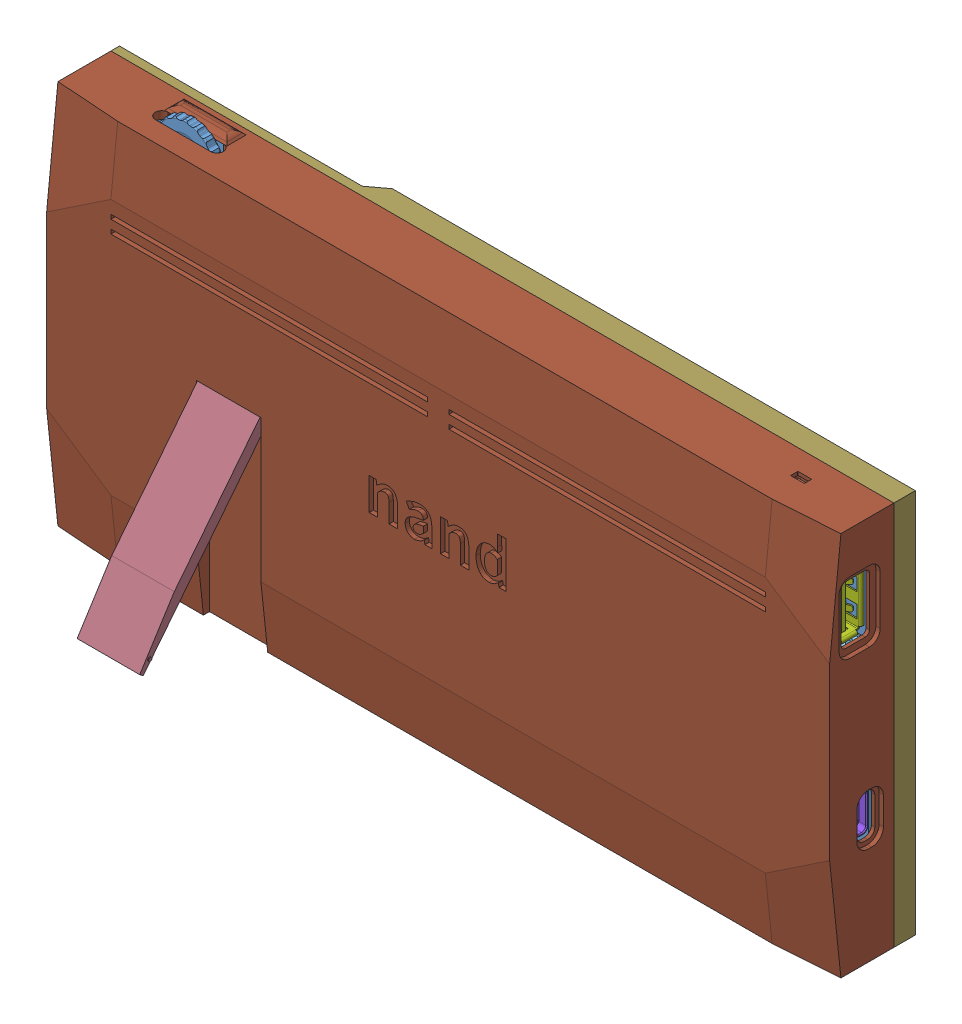
SolidWorks assembly model01, configuration 默认. Lengths in mm.
Overall size (182.71 95.18 52.67).
146 component instances, 34 part files, 28 mates.
Components (placement in the parent):
- Copy of CTR_PAD.step-1: Copy of CTR_PAD.step [默认] at (14.9481 50.9273 157.9259) size (178.7 93.18 19.65)
  - Board.step-1: Board.step [默认] at origin size (178.7 87.58 1.9)
    - Open CASCADE STEP translator 6.8 1.1.1.step-1: Open CASCADE STEP translator 6.8 1.1.1.step [默认] at (0 0 -1.9037) size (178.7 87.58 1.9)
  - K1_1.step-1: K1_1.step [默认] at origin size (7.8 3.6 3.5)
    - User_Library-E-Switch_-_TL3330AF130QG_(Tact_Switch,_SMD).step-1: User_Library-E-Switch_-_TL3330AF130QG_(Tact_Switch,_SMD).step [默认] at (168.6 -0.394 0) x (-1 0 0) z (0 1 0) size (7.8 3.5 3.6)
  - JP4.step-1: JP4.step [默认] at origin size (5.19 12.65 3.4)
    - MOLEX1.25-WS-6P.step-1: MOLEX1.25-WS-6P.step [默认] at (176.345 -30.9118 0) x (0 1 0) z (0 0 1) size (12.65 5.19 3.4)
      - MOLEX1.25-WS-____.step-1: MOLEX1.25-WS-____.step [默认] at (3.125 1.89 1.375) size (0.32 4.2 1.72)
      - MOLEX1.25-WS-____.step-2: MOLEX1.25-WS-____.step [默认] at (1.875 1.89 1.375) size (0.32 4.2 1.72)
      - MOLEX1.25-WS-____.step-3: MOLEX1.25-WS-____.step [默认] at (0.625 1.89 1.375) size (0.32 4.2 1.72)
      - MOLEX1.25-WS-____.step-4: MOLEX1.25-WS-____.step [默认] at (-0.625 1.89 1.375) size (0.32 4.2 1.72)
      - MOLEX1.25-WS-____.step-5: MOLEX1.25-WS-____.step [默认] at (-1.875 1.89 1.375) size (0.32 4.2 1.72)
      - MOLEX1.25-WS-____.step-6: MOLEX1.25-WS-____.step [默认] at (-3.125 1.89 1.375) size (0.32 4.2 1.72)
      - LOGO_0.25.step-1: LOGO_0.25.step [默认] at (3.4 -1.1304 0.195) size (0.75 0.87 0.01)
      - MOLEX1.25-WS-6P-0.step-1: MOLEX1.25-WS-6P-0.step [默认] at origin size (12.65 4.2 3.4)
  - USB1.step-1: USB1.step [默认] at origin size (14.7 15.5 7.95)
    - USB_A_______-__-2.step-1: USB_A_______-__-2.step [默认] at (168.4838 -16.002 0) x (0 1 0) z (0 0 1) size (15.5 14.7 7.95)
      - LOGO_.step-1: LOGO_.step [默认] at (0.0236 -0.0345 0.196) x (-1 0 0) z (0 0 -1) size (1.2 1.38 0.01)
      - USB_A_______-__-2-1.step-1: USB_A_______-__-2-1.step [默认] at origin size (15.5 14.7 7.95)
  - U8.step-1: U8.step [默认] at origin size (7.9 8.94 4.2)
    - USB_Type_C_Port_(SMD_Type)_RGB15724527.step-1: USB_Type_C_Port_(SMD_Type)_RGB15724527.step [默认] at (171.3143 -58.97 1.651) x (0 1 0) z (0 0 -1) size (8.94 7.9 4.2)
  - JP2.step-1: JP2.step [默认] at origin size (0.51 6.25 12)
    - DJ610-4.8x0.5x14.step-1: DJ610-4.8x0.5x14.step [默认] at (155.879 -80.1986 -1.9037) x (0 1 0) z (0 0 -1) size (6.25 0.51 12)
      - DJ610-4.8x0.5x14-2.step-1: DJ610-4.8x0.5x14-2.step [默认] at origin size (6.25 0.51 12)
      - LOGO_0.1.step-1: LOGO_0.1.step [默认] at (-0.0714 0.0198 0.048) size (0.3 0.35 0)
  - JP3.step-1: JP3.step [默认] at origin size (0.51 6.25 12)
    - DJ610-4.8x0.5x14.step-1: DJ610-4.8x0.5x14.step [默认] at (145.719 -80.1986 -1.9037) x (0 1 0) z (0 0 -1) size (6.25 0.51 12)
      - DJ610-4.8x0.5x14-2.step-1: DJ610-4.8x0.5x14-2.step [默认] at origin size (6.25 0.51 12)
      - LOGO_0.1.step-1: LOGO_0.1.step [默认] at (-0.0714 0.0198 0.048) size (0.3 0.35 0)
  - Designator10.step-1: Designator10.step [默认] at origin size (6.5 7.3 13.51)
    - SMA-KE-LI.step-1: SMA-KE-LI.step [默认] at (110.2469 -80.1989 -1.9037) x (-1 0 0) z (0 0 -1) size (6.5 7.3 13.5)
      - SMA-KE-LI-3.step-1: SMA-KE-LI-3.step [默认] at origin size (6.5 7.3 13.5)
      - LOGO_0.25-4.step-1: LOGO_0.25-4.step [默认] at (0.0036 0.0616 -3.1525) size (0.75 0.87 0.01)
  - Designator9.step-1: Designator9.step [默认] at origin size (6.5 7.3 13.51)
    - SMA-KE-LI.step-1: SMA-KE-LI.step [默认] at (82.0269 -80.1369 -1.9037) x (-1 0 0) z (0 0 -1) size (6.5 7.3 13.5)
      - SMA-KE-LI-3.step-1: SMA-KE-LI-3.step [默认] at origin size (6.5 7.3 13.5)
      - LOGO_0.25-4.step-1: LOGO_0.25-4.step [默认] at (0.0036 0.0616 -3.1525) size (0.75 0.87 0.01)
  - R3.step-1: R3.step [默认] at origin size (1.6 0.8 0.4)
    - R_0603.step-1: R_0603.step [默认] at (50.1906 -13.906 -1.9037) x (-1 0 0) z (0 0 -1) size (1.6 0.8 0.4)
      - R_0603-5.step-1: R_0603-5.step [默认] at origin size (1.6 0.8 0.4)
      - LOGO_-6.step-1: LOGO_-6.step [默认] at (0.0001 0.0322 -0.0016) x (-1 0 0) z (0 0 -1) size (0.48 0.55 0)
  - KEY4.step-1: KEY4.step [默认] at origin size (10.71 10 7.1)
    - 43447.step-1: 43447.step [默认] at (38.778 -26.673 -1.9037) x (1 0 0) z (0 1 0) size (10.71 7.1 10)
  - KEY3.step-1: KEY3.step [默认] at origin size (10.71 10 7.1)
    - 43447.step-1: 43447.step [默认] at (38.778 -41.833 -1.9037) x (1 0 0) z (0 1 0) size (10.71 7.1 10)
  - KEY2.step-1: KEY2.step [默认] at origin size (10.71 10 7.1)
    - 43447.step-1: 43447.step [默认] at (38.778 -56.993 -1.9037) x (1 0 0) z (0 1 0) size (10.71 7.1 10)
  - KEY1.step-1: KEY1.step [默认] at origin size (10.71 10 7.1)
    - 43447.step-1: 43447.step [默认] at (38.778 -72.153 -1.9037) x (1 0 0) z (0 1 0) size (10.71 7.1 10)
  - S1.step-1: S1.step [默认] at origin size (19.75 19.71 4.5)
    - SIQ-02FVS3.step-1: SIQ-02FVS3.step [默认] at (23.5 -2.4777 2) x (1 0 0) z (0 -1 0) size (19.75 4.5 19.71)
      - SIQ_BASE_ASM.step-1: SIQ_BASE_ASM.step [默认] at origin size (10.6 2.2 11.36)
      - SIQ_COVER.step-1: SIQ_COVER.step [默认] at origin size (10.45 2.3 11.25)
      - SIQ_ROTOR_ASM.step-1: SIQ_ROTOR_ASM.step [默认] at (0 0.25 0) size (4.63 1.1 4.26)
      - DIAL_KNOB.step-1: DIAL_KNOB.step [默认] at (0 0.3 0) x (0.866025 0 0.5) z (-0.5 0 0.866025) size (14.5 2.18 14.38)
  - R1.step-1: R1.step [默认] at origin size (1.6 0.8 0.4)
    - R_0603.step-1: R_0603.step [默认] at (50.1906 -15.557 -1.9037) x (-1 0 0) z (0 0 -1) size (1.6 0.8 0.4)
      - R_0603-5.step-1: R_0603-5.step [默认] at origin size (1.6 0.8 0.4)
      - LOGO_-6.step-1: LOGO_-6.step [默认] at (0.0001 0.0322 -0.0016) x (-1 0 0) z (0 0 -1) size (0.48 0.55 0)
  - LED1.step-1: LED1.step [默认] at origin size (3.5 2.8 1.91)
    - LED_3528-4Pin_____.step-1: LED_3528-4Pin_____.step [默认] at (50.1905 -11.4876 -1.9037) x (1 0 0) z (0 0 -1) size (3.5 2.8 1.91)
      - LOGO_0.25-7.step-1: LOGO_0.25-7.step [默认] at (-0.0099 0 0.0475) x (0 -1 0) z (0 0 -1) size (0.75 0.87 0.01)
      - LED_3528-4Pin_____-8.step-1: LED_3528-4Pin_____-8.step [默认] at origin size (3.5 2.8 1.9)
  - R4.step-1: R4.step [默认] at origin size (1.6 0.8 0.4)
    - R_0603.step-1: R_0603.step [默认] at (50 -26 -1.9037) x (1 0 0) z (0 0 -1) size (1.6 0.8 0.4)
      - R_0603-5.step-1: R_0603-5.step [默认] at origin size (1.6 0.8 0.4)
      - LOGO_-6.step-1: LOGO_-6.step [默认] at (0.0001 0.0322 -0.0016) x (-1 0 0) z (0 0 -1) size (0.48 0.55 0)
  - LED3.step-1: LED3.step [默认] at origin size (2 1.25 0.67)
    - LED_0805-Y.step-1: LED_0805-Y.step [默认] at (50.0001 -23.9998 -1.9037) x (-1 0 0) z (0 0 -1) size (2 1.25 0.67)
      - LOGO_-9.step-1: LOGO_-9.step [默认] at (0 0.0303 -0.002) x (-1 0 0) z (0 0 -1) size (0.6 0.69 0)
      - LED_0805-Y-10.step-1: LED_0805-Y-10.step [默认] at origin size (2 1.25 0.67)
  - K5.step-1: K5.step [默认] at origin size (9 6 4.2)
    - TSW_SMD-6x6x4.3.step-1: TSW_SMD-6x6x4.3.step [默认] at (10 -26.8 -1.9537) x (0 -1 0) z (1 0 0) size (6 4.2 9)
      - LOGO_-11.step-1: LOGO_-11.step [默认] at (0.0186 0.396 1.2756) x (1 0 0) z (0 -1 0) size (1.2 1.38 0.01)
      - TSW_SMD-6x6x4.3-12.step-1: TSW_SMD-6x6x4.3-12.step [默认] at origin size (6 4.2 9)
  - K8.step-1: K8.step [默认] at origin size (9 6 4.2)
    - TSW_SMD-6x6x4.3.step-1: TSW_SMD-6x6x4.3.step [默认] at (23.5 -72.2164 -1.9537) x (0 -1 0) z (1 0 0) size (6 4.2 9)
      - LOGO_-11.step-1: LOGO_-11.step [默认] at (0.0186 0.396 1.2756) x (1 0 0) z (0 -1 0) size (1.2 1.38 0.01)
      - TSW_SMD-6x6x4.3-12.step-1: TSW_SMD-6x6x4.3-12.step [默认] at origin size (6 4.2 9)
  - K7.step-1: K7.step [默认] at origin size (9 6 4.2)
    - TSW_SMD-6x6x4.3.step-1: TSW_SMD-6x6x4.3.step [默认] at (23.5 -57.0564 -1.9537) x (0 -1 0) z (1 0 0) size (6 4.2 9)
      - LOGO_-11.step-1: LOGO_-11.step [默认] at (0.0186 0.396 1.2756) x (1 0 0) z (0 -1 0) size (1.2 1.38 0.01)
      - TSW_SMD-6x6x4.3-12.step-1: TSW_SMD-6x6x4.3-12.step [默认] at origin size (6 4.2 9)
  - R9.step-1: R9.step [默认] at origin size (1.6 0.8 0.4)
    - R_0603.step-1: R_0603.step [默认] at (50.1906 -74.216 -1.9037) x (1 0 0) z (0 0 -1) size (1.6 0.8 0.4)
      - R_0603-5.step-1: R_0603-5.step [默认] at origin size (1.6 0.8 0.4)
      - LOGO_-6.step-1: LOGO_-6.step [默认] at (0.0001 0.0322 -0.0016) x (-1 0 0) z (0 0 -1) size (0.48 0.55 0)
  - R8.step-1: R8.step [默认] at origin size (1.6 0.8 0.4)
    - R_0603.step-1: R_0603.step [默认] at (50.0634 -59.056 -1.9037) x (1 0 0) z (0 0 -1) size (1.6 0.8 0.4)
      - R_0603-5.step-1: R_0603-5.step [默认] at origin size (1.6 0.8 0.4)
      - LOGO_-6.step-1: LOGO_-6.step [默认] at (0.0001 0.0322 -0.0016) x (-1 0 0) z (0 0 -1) size (0.48 0.55 0)
  - R6.step-1: R6.step [默认] at origin size (1.6 0.8 0.4)
    - R_0603.step-1: R_0603.step [默认] at (50.1906 -43.896 -1.9037) x (1 0 0) z (0 0 -1) size (1.6 0.8 0.4)
      - R_0603-5.step-1: R_0603-5.step [默认] at origin size (1.6 0.8 0.4)
      - LOGO_-6.step-1: LOGO_-6.step [默认] at (0.0001 0.0322 -0.0016) x (-1 0 0) z (0 0 -1) size (0.48 0.55 0)
  - R2.step-1: R2.step [默认] at origin size (1.6 0.8 0.4)
    - R_0603.step-1: R_0603.step [默认] at (50 -31.473 -1.9037) x (1 0 0) z (0 0 -1) size (1.6 0.8 0.4)
      - R_0603-5.step-1: R_0603-5.step [默认] at origin size (1.6 0.8 0.4)
      - LOGO_-6.step-1: LOGO_-6.step [默认] at (0.0001 0.0322 -0.0016) x (-1 0 0) z (0 0 -1) size (0.48 0.55 0)
  - LED6.step-1: LED6.step [默认] at origin size (2 1.25 0.67)
    - LED_0805-R.step-1: LED_0805-R.step [默认] at (50 -72.2163 -1.9037) x (-1 0 0) z (0 0 -1) size (2 1.25 0.67)
      - LOGO_-13.step-1: LOGO_-13.step [默认] at (0 0.0303 -0.002) x (-1 0 0) z (0 0 -1) size (0.6 0.69 0)
      - LED_0805-R-14.step-1: LED_0805-R-14.step [默认] at origin size (2 1.25 0.67)
  - LED5.step-1: LED5.step [默认] at origin size (2 1.25 0.67)
    - LED_0805-R.step-1: LED_0805-R.step [默认] at (50 -57.0563 -1.9037) x (-1 0 0) z (0 0 -1) size (2 1.25 0.67)
      - LOGO_-13.step-1: LOGO_-13.step [默认] at (0 0.0303 -0.002) x (-1 0 0) z (0 0 -1) size (0.6 0.69 0)
      - LED_0805-R-14.step-1: LED_0805-R-14.step [默认] at origin size (2 1.25 0.67)
  - LED4.step-1: LED4.step [默认] at origin size (2 1.25 0.67)
    - LED_0805-R.step-1: LED_0805-R.step [默认] at (50 -41.8963 -1.9037) x (-1 0 0) z (0 0 -1) size (2 1.25 0.67)
      - LOGO_-13.step-1: LOGO_-13.step [默认] at (0 0.0303 -0.002) x (-1 0 0) z (0 0 -1) size (0.6 0.69 0)
      - LED_0805-R-14.step-1: LED_0805-R-14.step [默认] at origin size (2 1.25 0.67)
  - LED2.step-1: LED2.step [默认] at origin size (2 1.25 0.67)
    - LED_0805-Y.step-1: LED_0805-Y.step [默认] at (50.0001 -29.473 -1.9037) x (-1 0 0) z (0 0 -1) size (2 1.25 0.67)
      - LOGO_-9.step-1: LOGO_-9.step [默认] at (0 0.0303 -0.002) x (-1 0 0) z (0 0 -1) size (0.6 0.69 0)
      - LED_0805-Y-10.step-1: LED_0805-Y-10.step [默认] at origin size (2 1.25 0.67)
  - K6.step-1: K6.step [默认] at origin size (9 6 4.2)
    - TSW_SMD-6x6x4.3.step-1: TSW_SMD-6x6x4.3.step [默认] at (23.5 -41.96 -1.9537) x (0 -1 0) z (1 0 0) size (6 4.2 9)
      - LOGO_-11.step-1: LOGO_-11.step [默认] at (0.0186 0.396 1.2756) x (1 0 0) z (0 -1 0) size (1.2 1.38 0.01)
      - TSW_SMD-6x6x4.3-12.step-1: TSW_SMD-6x6x4.3-12.step [默认] at origin size (6 4.2 9)
  - K4.step-1: K4.step [默认] at origin size (9 6 4.2)
    - TSW_SMD-6x6x4.3.step-1: TSW_SMD-6x6x4.3.step [默认] at (23.5 -26.8 -1.9537) x (0 -1 0) z (1 0 0) size (6 4.2 9)
      - LOGO_-11.step-1: LOGO_-11.step [默认] at (0.0186 0.396 1.2756) x (1 0 0) z (0 -1 0) size (1.2 1.38 0.01)
      - TSW_SMD-6x6x4.3-12.step-1: TSW_SMD-6x6x4.3-12.step [默认] at origin size (6 4.2 9)
  - K2.step-1: K2.step [默认] at origin size (9 6 4.2)
    - TSW_SMD-6x6x4.3.step-1: TSW_SMD-6x6x4.3.step [默认] at (38.7779 -11.64 -1.9537) x (0 -1 0) z (1 0 0) size (6 4.2 9)
      - LOGO_-11.step-1: LOGO_-11.step [默认] at (0.0186 0.396 1.2756) x (1 0 0) z (0 -1 0) size (1.2 1.38 0.01)
      - TSW_SMD-6x6x4.3-12.step-1: TSW_SMD-6x6x4.3-12.step [默认] at origin size (6 4.2 9)
  - K3.step-1: K3.step [默认] at origin size (9 6 4.2)
    - TSW_SMD-6x6x4.3.step-1: TSW_SMD-6x6x4.3.step [默认] at (23.5 -11.64 -1.9537) x (0 -1 0) z (1 0 0) size (6 4.2 9)
      - LOGO_-11.step-1: LOGO_-11.step [默认] at (0.0186 0.396 1.2756) x (1 0 0) z (0 -1 0) size (1.2 1.38 0.01)
      - TSW_SMD-6x6x4.3-12.step-1: TSW_SMD-6x6x4.3-12.step [默认] at origin size (6 4.2 9)
  - K1.step-1: K1.step [默认] at origin size (9 6 4.2)
    - TSW_SMD-6x6x4.3.step-1: TSW_SMD-6x6x4.3.step [默认] at (10 -11.64 -1.9537) x (0 -1 0) z (1 0 0) size (6 4.2 9)
      - LOGO_-11.step-1: LOGO_-11.step [默认] at (0.0186 0.396 1.2756) x (1 0 0) z (0 -1 0) size (1.2 1.38 0.01)
      - TSW_SMD-6x6x4.3-12.step-1: TSW_SMD-6x6x4.3-12.step [默认] at origin size (6 4.2 9)
- 零件28^model01-1: 零件28^model01 [默认] at (14.9481 50.9273 156.0222) x (-1 0 0) z (0 0 -1) size (178.7 85.8 2) (virtual)
- 零件31^model01-1: 零件31^model01 [默认] at (14.9481 50.9273 156.0222) size (182.71 90.8 15) (virtual)
- 装配体1^model01-1: 装配体1^model01 [默认] at origin (virtual)
- 零件32^model01-1: 零件32^model01 [默认] at (14.9481 50.9273 154.0222) x (-1 0 0) z (0 0 -1) size (182.7 89.8 7) (virtual)
- PANNEL-BOARD-1: PANNEL-BOARD [默认] at (14.9481 50.9273 151.4589) size (58 85.8 1.69) (hidden)
  - pannel-1: pannel [默认] at origin size (58 85.8 1.69)
    - Board-Part-1-1: Board-Part-1 [默认] at (0 0 -1.6914) size (58 85.8 1.69)
- 零件1^model01-1: 零件1^model01 [默认] at (14.9481 50.9273 152.0222) x (-1 0 0) z (0 0 -1) size (120.9 76 4.03) (hidden, virtual)
- 按键帽^model01-1: 按键帽^model01 [默认] at (14.9481 50.9273 156.0222) x (-1 0 0) z (0 0 -1) size (12.5 12.5 10.2) (hidden, virtual)
- 零件3^model01-2: 零件3^model01 [默认] at (47.9481 49.4661 151.8244) x (0 -0.620915 -0.783878) z (1 0 0) size (2.6 49.3 20)
- 按键帽^model01-2: 按键帽^model01 [默认] at (80.3991 47.8093 156.0222) x (0 1 0) z (0 0 -1) size (12.5 12.5 10.2) (hidden, virtual)
Mates (geometry in assembly coordinates):
- 在位1: in place: plane of ? through (14.9481 -34.8727 156.0222) normal (0 0 -1); plane of ? through (0 0 156.0222) normal (0 0 -1); moOrthogonalPlaneRef_w of ? through (14.9481 -34.8727 156.0222) normal (0 0 -1); plane of ? through (0 0 156.0222) normal (0 1 0); plane of ? through (14.9481 -34.8727 156.0222) normal (0 0 -1); plane of ? through (0 0 156.0222) normal (-1 0 0); plane of ? through (14.9481 -34.8727 156.0222) normal (0 0 -1); unknown of ?
- 重合1: coincident aligned: plane of ?; plane of ?
- 重合2: coincident aligned: moOrthogonalPlaneRef_w of Copy of CTR_PAD.step-1/Board.step-1/Open CASCADE STEP translator 6.8 1.1.1.step-1 through (14.9481 50.9273 156.0222) normal (0 1 0); plane of 零件28^装配体1-1 through (14.9481 50.9273 156.0222) normal (0 1 0)
- 重合3: coincident anti-aligned: moOrthogonalPlaneRef_w of Copy of CTR_PAD.step-1/Board.step-1/Open CASCADE STEP translator 6.8 1.1.1.step-1 through (14.9481 50.9273 156.0222) normal (1 0 0); plane of 零件28^装配体1-1 through (14.9481 50.9273 156.0222) normal (-1 0 0)
- 在位2: in place: plane of ? through (14.9481 50.9273 156.0222) normal (0 0 1); plane of ? through (0 0 156.0222) normal (0 0 1); plane of ? through (14.9481 50.9273 156.0222) normal (0 0 1); plane of ? through (0 0 156.0222) normal (0 1 0); plane of ? through (14.9481 50.9273 156.0222) normal (0 0 1); plane of ? through (0 0 156.0222) normal (1 0 0); plane of ? through (14.9481 50.9273 156.0222) normal (0 0 1); unknown of ?
- 重合1: coincident aligned: plane of ?; plane of ?
- 重合2: coincident aligned: moOrthogonalPlaneRef_w of 零件28^装配体1-1 through (14.9481 50.9273 156.0222) normal (0 1 0); plane of 零件31^model01-1 through (14.9481 50.9273 156.0222) normal (0 1 0)
- 重合3: coincident anti-aligned: moOrthogonalPlaneRef_w of 零件28^装配体1-1 through (14.9481 50.9273 156.0222) normal (-1 0 0); plane of 零件31^model01-1 through (14.9481 50.9273 156.0222) normal (1 0 0)
- 在位3: in place: plane of ? through (14.9481 50.9273 154.0222) normal (0 0 -1); plane of ? through (0 0 154.0222) normal (0 0 -1); plane of ? through (14.9481 50.9273 154.0222) normal (0 0 -1); plane of ? through (0 0 154.0222) normal (0 1 0); plane of ? through (14.9481 50.9273 154.0222) normal (0 0 -1); plane of ? through (0 0 154.0222) normal (-1 0 0); plane of ? through (14.9481 50.9273 154.0222) normal (0 0 -1); unknown of 零件32^model01-1
- 重合1: coincident aligned: plane of ?; plane of ?
- 重合2: coincident aligned: moOrthogonalPlaneRef_w of 零件28^装配体1-1 through (14.9481 50.9273 154.0222) normal (0 1 0); plane of 零件32^model01-1 through (14.9481 50.9273 154.0222) normal (0 1 0)
- 重合3: coincident anti-aligned: moOrthogonalPlaneRef_w of 零件28^装配体1-1 through (14.9481 50.9273 154.0222) normal (1 0 0); plane of 零件32^model01-1 through (14.9481 50.9273 154.0222) normal (-1 0 0)
- 同心1: concentric anti-aligned: circle of 零件28^装配体1-1; circle of PANNEL-BOARD-1/pannel-1/Board-Part-1-1
- 同心2: concentric anti-aligned: circle of 零件28^装配体1-1; circle of PANNEL-BOARD-1/pannel-1/Board-Part-1-1
- 在位4: in place: plane of 零件32^model01-1 through (14.9481 50.9273 152.0222) normal (0 0 -1); plane of ? through (0 0 152.0222) normal (0 0 -1); plane of 零件32^model01-1 through (14.9481 50.9273 152.0222) normal (0 0 -1); plane of ? through (0 0 152.0222) normal (0 1 0); plane of 零件32^model01-1 through (14.9481 50.9273 152.0222) normal (0 0 -1); plane of ? through (0 0 152.0222) normal (-1 0 0); plane of 零件32^model01-1 through (14.9481 50.9273 152.0222) normal (0 0 -1); unknown of 零件1^model01-1
- 重合7: coincident aligned: plane of ?; plane of ?
- 重合8: coincident aligned: moOrthogonalPlaneRef_w of 零件32^model01-1 through (14.9481 50.9273 152.0222) normal (0 1 0); plane of 零件1^model01-1 through (14.9481 50.9273 152.0222) normal (0 1 0)
- 重合9: coincident anti-aligned: moOrthogonalPlaneRef_w of 零件32^model01-1 through (14.9481 50.9273 152.0222) normal (1 0 0); plane of 零件1^model01-1 through (14.9481 50.9273 152.0222) normal (-1 0 0)
- 在位6: in place: plane of ? through (14.9481 -34.8727 156.0222) normal (0 0 -1); plane of ? through (0 0 156.0222) normal (0 0 -1); plane of ? through (14.9481 -34.8727 156.0222) normal (0 0 -1); plane of ? through (0 0 156.0222) normal (0 1 0); plane of ? through (14.9481 -34.8727 156.0222) normal (0 0 -1); plane of ? through (0 0 156.0222) normal (-1 0 0); plane of ? through (14.9481 -34.8727 156.0222) normal (0 0 -1); unknown of ?
- 重合11: coincident aligned: plane of ?; plane of ?
- 重合12: coincident aligned: moOrthogonalPlaneRef_w of Copy of CTR_PAD.step-1/Board.step-1/Open CASCADE STEP translator 6.8 1.1.1.step-1 through (14.9481 50.9273 156.0222) normal (0 1 0); plane of 零件3^model01-1 through (14.9481 50.9273 156.0222) normal (0 1 0)
- 重合13: coincident anti-aligned: moOrthogonalPlaneRef_w of Copy of CTR_PAD.step-1/Board.step-1/Open CASCADE STEP translator 6.8 1.1.1.step-1 through (14.9481 50.9273 156.0222) normal (1 0 0); plane of 零件3^model01-1 through (14.9481 50.9273 156.0222) normal (-1 0 0)
- 重合13: coincident aligned: plane of 零件31^model01-1 through (55.4481 50.9273 156.0222) normal (-1 0 0); plane of 零件3^model01-2 through (55.4481 49.4661 151.8244) normal (-1 0 0)
- 同心3: concentric anti-aligned: cylinder of 零件31^model01-1 through (44.4481 11.1273 167.5222) axis (1 0 0) radius 0.75; circle of 零件3^model01-2
- LimitDistance2: limit distance = 0 mm: plane of 零件3^model01-2 through (62.7481 11.9344 168.5412) normal (0 0.620915 0.783878); line of 零件31^model01-1 through (47.9481 11.3273 169.0222) axis (1 0 0)
- 同心4: concentric anti-aligned: circle of PANNEL-BOARD-1/pannel-1/Board-Part-1-1; circle of 按键帽^model01-2
- 平行2: parallel anti-aligned: line of 零件32^model01-1 through (69.6148 52.9273 152.0222) axis (-1 0 0); line of 按键帽^model01-2 through (47.9761 15.2813 152.8222) axis (1 0 0)
- 重合21: coincident anti-aligned: plane of Copy of CTR_PAD.step-1/Board.step-1/Open CASCADE STEP translator 6.8 1.1.1.step-1 through (14.9481 -34.8727 156.0222) normal (0 0 -1); plane of 按键帽^model01-2 through (80.3991 47.8093 156.0222) normal (0 0 1)
